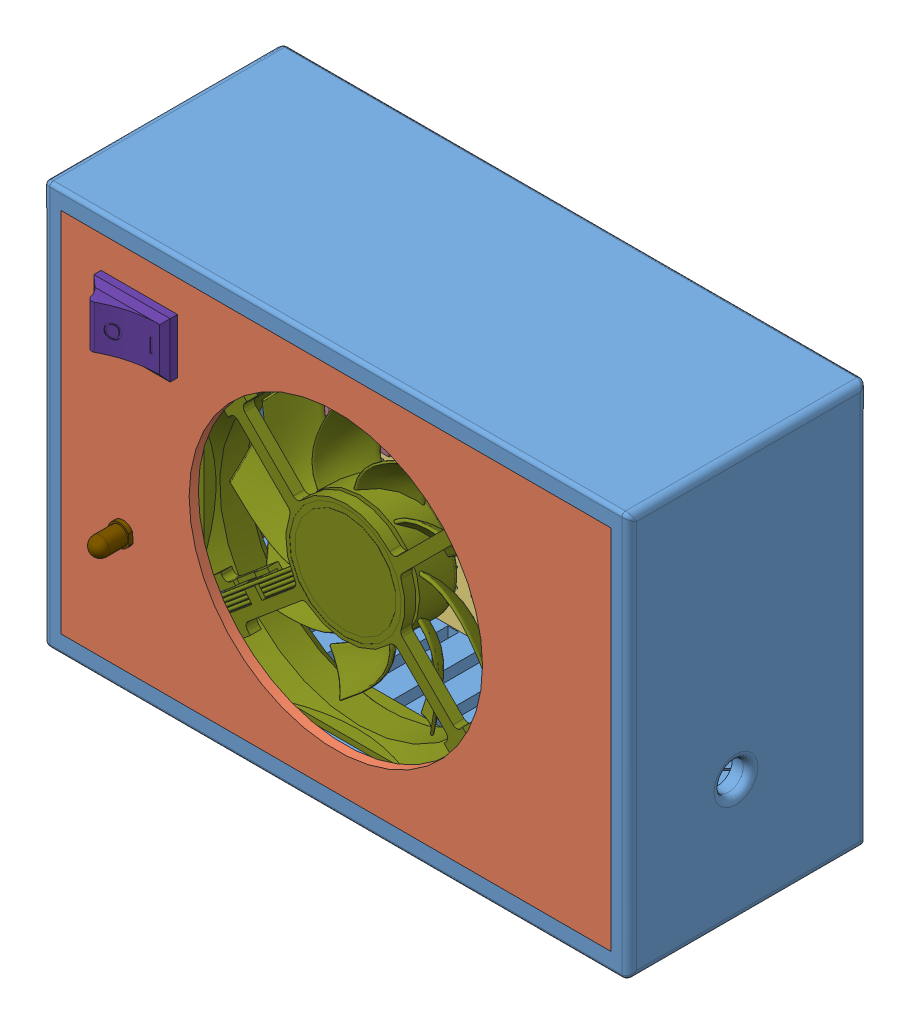
SolidWorks assembly Assem1 final, configuration Default. Lengths in mm.
Overall size (160 110 73.7).
688 component instances, 72 part files, 18 mates.
Components (placement in the parent):
- Lead acid charger_enclosure-2: Lead acid charger_enclosure [Default] at origin size (160 110 65)
- Part2-3: Part2 [Default] at (0 0 60) x (0 0 -1) z (1 0 0) size (42.25 100 150)
- PCB2.step-2: PCB2.step [Default] at (-67.4243 -42.9166 12.1575) size (119 88 45.91)
  - Board.step-1: Board.step [Default] at origin size (119 88 0.41)
    - Open CASCADE STEP translator 6.8 2.1.1.step-1: Open CASCADE STEP translator 6.8 2.1.1.step [Default] at (0 0 -0.4115) size (119 88 0.41)
  - D3.step-1: D3.step [Default] at origin size (2.72 10.58 4.72)
    - 5897140976.step-1: 5897140976.step [Default] at (24 47.5001 -2) x (0 1 0) z (0 0 1) size (2.29 2.29 1.52)
      - Cylinder.step-1: Cylinder.step [Default] at origin size (2.29 2.29 1.52)
    - 5897140736.step-1: 5897140736.step [Default] at (24 47.5001 1.36) x (0 1 0) z (0 0 1) size (0.86 0.86 0.86)
      - Sphere.step-1: Sphere.step [Default] at origin size (0.86 0.86 0.86)
    - 5897140496.step-1: 5897140496.step [Default] at (24 40.4001 1.36) x (0 0 -1) z (0 1 0) size (2.72 2.72 5.2)
      - Cylinder-0.step-1: Cylinder-0.step [Default] at origin size (2.72 2.72 5.2)
    - 5897140256.step-1: 5897140256.step [Default] at (24 45.6 1.36) x (0 0 -1) z (0 1 0) size (0.86 0.86 1.9)
      - Cylinder-1.step-1: Cylinder-1.step [Default] at origin size (0.86 0.86 1.9)
    - 5897140096.step-1: 5897140096.step [Default] at (24 40.4 1.36) x (0 0 -1) z (0 -1 0) size (0.86 0.86 1.9)
      - Cylinder-2.step-1: Cylinder-2.step [Default] at origin size (0.86 0.86 1.9)
    - 5897139936.step-1: 5897139936.step [Default] at (24 38.4999 1.36) x (0 -1 0) z (0 0 1) size (0.86 0.86 0.86)
      - Sphere-3.step-1: Sphere-3.step [Default] at origin size (0.86 0.86 0.86)
    - 5897139776.step-1: 5897139776.step [Default] at (24 38.4999 -2) x (0 -1 0) z (0 0 1) size (0.86 0.86 3.36)
      - Cylinder-4.step-1: Cylinder-4.step [Default] at origin size (0.86 0.86 3.36)
  - D1.step-1: D1.step [Default] at origin size (5.6 16.87 20.27)
    - 5790703040.step-1: 5790703040.step [Default] at (71 42 0) x (0 -1 0) z (-1 0 0) size (16.87 20.27 5.6)
  - D2.step-1: D2.step [Default] at origin size (16.87 5.6 20.27)
    - 5790703360.step-1: 5790703360.step [Default] at (79 78 0) x (-1 0 0) z (0 1 0) size (16.87 20.27 5.6)
  - U8.step-1: U8.step [Default] at origin size (7.89 10.15 6.68)
    - 5985638288.step-1: 5985638288.step [Default] at (35.891 41.689 0.51) size (6.6 10.15 4.57)
      - Extruded-5.step-1: Extruded-5.step [Default] at origin size (6.6 10.15 4.57)
    - 5985638128.step-1: 5985638128.step [Default] at (39.701 45.499 -1.6) size (0.27 0.72 1.6)
      - Extruded-2.step-1: Extruded-2.step [Default] at origin size (0.27 0.72 1.6)
    - 5985637968.step-1: 5985637968.step [Default] at (39.5135 45.499 2.66) size (0.64 1 0.27)
      - Extruded-3.step-1: Extruded-3.step [Default] at origin size (0.64 1 0.27)
    - 5985637808.step-1: 5985637808.step [Default] at (39.701 45.499 0) size (0.27 1 2.66)
      - Extruded-4.step-1: Extruded-4.step [Default] at origin size (0.27 1 2.66)
    - 5985638128.step-2: 5985638128.step [Default] at (39.701 42.959 -1.6) size (0.27 0.72 1.6)
      - Extruded-2.step-1: Extruded-2.step [Default] at origin size (0.27 0.72 1.6)
    - 5985637968.step-2: 5985637968.step [Default] at (39.5135 42.959 2.66) size (0.64 1 0.27)
      - Extruded-3.step-1: Extruded-3.step [Default] at origin size (0.64 1 0.27)
    - 5985637808.step-2: 5985637808.step [Default] at (39.701 42.959 0) size (0.27 1 2.66)
      - Extruded-4.step-1: Extruded-4.step [Default] at origin size (0.27 1 2.66)
    - 5985638128.step-3: 5985638128.step [Default] at (39.701 40.419 -1.6) size (0.27 0.72 1.6)
      - Extruded-2.step-1: Extruded-2.step [Default] at origin size (0.27 0.72 1.6)
    - 5985637968.step-3: 5985637968.step [Default] at (39.5135 40.419 2.66) size (0.64 1 0.27)
      - Extruded-3.step-1: Extruded-3.step [Default] at origin size (0.64 1 0.27)
    - 5985637808.step-3: 5985637808.step [Default] at (39.701 40.419 0) size (0.27 1 2.66)
      - Extruded-4.step-1: Extruded-4.step [Default] at origin size (0.27 1 2.66)
    - 5985638128.step-4: 5985638128.step [Default] at (39.701 37.879 -1.6) size (0.27 0.72 1.6)
      - Extruded-2.step-1: Extruded-2.step [Default] at origin size (0.27 0.72 1.6)
    - 5985637968.step-4: 5985637968.step [Default] at (39.5135 37.879 2.66) size (0.64 1 0.27)
      - Extruded-3.step-1: Extruded-3.step [Default] at origin size (0.64 1 0.27)
    - 5985637808.step-4: 5985637808.step [Default] at (39.701 37.879 0) size (0.27 1 2.66)
      - Extruded-4.step-1: Extruded-4.step [Default] at origin size (0.27 1 2.66)
    - 5985638128.step-5: 5985638128.step [Default] at (32.081 37.879 -1.6) size (0.27 0.72 1.6)
      - Extruded-2.step-1: Extruded-2.step [Default] at origin size (0.27 0.72 1.6)
    - 5985637968.step-5: 5985637968.step [Default] at (32.2685 37.879 2.66) size (0.64 1 0.27)
      - Extruded-3.step-1: Extruded-3.step [Default] at origin size (0.64 1 0.27)
    - 5985637808.step-5: 5985637808.step [Default] at (32.081 37.879 0) size (0.27 1 2.66)
      - Extruded-4.step-1: Extruded-4.step [Default] at origin size (0.27 1 2.66)
    - 5985638128.step-6: 5985638128.step [Default] at (32.081 40.419 -1.6) size (0.27 0.72 1.6)
      - Extruded-2.step-1: Extruded-2.step [Default] at origin size (0.27 0.72 1.6)
    - 5985637968.step-6: 5985637968.step [Default] at (32.2685 40.419 2.66) size (0.64 1 0.27)
      - Extruded-3.step-1: Extruded-3.step [Default] at origin size (0.64 1 0.27)
    - 5985637808.step-6: 5985637808.step [Default] at (32.081 40.419 0) size (0.27 1 2.66)
      - Extruded-4.step-1: Extruded-4.step [Default] at origin size (0.27 1 2.66)
    - 5985638128.step-7: 5985638128.step [Default] at (32.081 42.959 -1.6) size (0.27 0.72 1.6)
      - Extruded-2.step-1: Extruded-2.step [Default] at origin size (0.27 0.72 1.6)
    - 5985637968.step-7: 5985637968.step [Default] at (32.2685 42.959 2.66) size (0.64 1 0.27)
      - Extruded-3.step-1: Extruded-3.step [Default] at origin size (0.64 1 0.27)
    - 5985637808.step-7: 5985637808.step [Default] at (32.081 42.959 0) size (0.27 1 2.66)
      - Extruded-4.step-1: Extruded-4.step [Default] at origin size (0.27 1 2.66)
    - 5985638128.step-8: 5985638128.step [Default] at (32.081 45.499 -1.6) size (0.27 0.72 1.6)
      - Extruded-2.step-1: Extruded-2.step [Default] at origin size (0.27 0.72 1.6)
    - 5985637968.step-8: 5985637968.step [Default] at (32.2685 45.499 2.66) size (0.64 1 0.27)
      - Extruded-3.step-1: Extruded-3.step [Default] at origin size (0.64 1 0.27)
    - 5985637808.step-8: 5985637808.step [Default] at (32.081 45.499 0) size (0.27 1 2.66)
      - Extruded-4.step-1: Extruded-4.step [Default] at origin size (0.27 1 2.66)
  - U9.step-1: U9.step [Default] at origin size (7.89 19.7 6.68)
    - 5985054240.step-1: 5985054240.step [Default] at (35.764 14.13 0.51) size (6.6 19.7 4.57)
      - Extruded-1.step-1: Extruded-1.step [Default] at origin size (6.6 19.7 4.57)
    - 5985638128.step-1: 5985638128.step [Default] at (39.574 23.02 -1.6) size (0.27 0.72 1.6)
      - Extruded-2.step-1: Extruded-2.step [Default] at origin size (0.27 0.72 1.6)
    - 5985637968.step-1: 5985637968.step [Default] at (39.3865 23.02 2.66) size (0.64 1 0.27)
      - Extruded-3.step-1: Extruded-3.step [Default] at origin size (0.64 1 0.27)
    - 5985637808.step-1: 5985637808.step [Default] at (39.574 23.02 0) size (0.27 1 2.66)
      - Extruded-4.step-1: Extruded-4.step [Default] at origin size (0.27 1 2.66)
    - 5985638128.step-2: 5985638128.step [Default] at (39.574 20.48 -1.6) size (0.27 0.72 1.6)
      - Extruded-2.step-1: Extruded-2.step [Default] at origin size (0.27 0.72 1.6)
    - 5985637968.step-2: 5985637968.step [Default] at (39.3865 20.48 2.66) size (0.64 1 0.27)
      - Extruded-3.step-1: Extruded-3.step [Default] at origin size (0.64 1 0.27)
    - 5985637808.step-2: 5985637808.step [Default] at (39.574 20.48 0) size (0.27 1 2.66)
      - Extruded-4.step-1: Extruded-4.step [Default] at origin size (0.27 1 2.66)
    - 5985638128.step-3: 5985638128.step [Default] at (39.574 17.94 -1.6) size (0.27 0.72 1.6)
      - Extruded-2.step-1: Extruded-2.step [Default] at origin size (0.27 0.72 1.6)
    - 5985637968.step-3: 5985637968.step [Default] at (39.3865 17.94 2.66) size (0.64 1 0.27)
      - Extruded-3.step-1: Extruded-3.step [Default] at origin size (0.64 1 0.27)
    - 5985637808.step-3: 5985637808.step [Default] at (39.574 17.94 0) size (0.27 1 2.66)
      - Extruded-4.step-1: Extruded-4.step [Default] at origin size (0.27 1 2.66)
    - 5985638128.step-4: 5985638128.step [Default] at (39.574 15.4 -1.6) size (0.27 0.72 1.6)
      - Extruded-2.step-1: Extruded-2.step [Default] at origin size (0.27 0.72 1.6)
    - 5985637968.step-4: 5985637968.step [Default] at (39.3865 15.4 2.66) size (0.64 1 0.27)
      - Extruded-3.step-1: Extruded-3.step [Default] at origin size (0.64 1 0.27)
    - 5985637808.step-4: 5985637808.step [Default] at (39.574 15.4 0) size (0.27 1 2.66)
      - Extruded-4.step-1: Extruded-4.step [Default] at origin size (0.27 1 2.66)
    - 5985638128.step-5: 5985638128.step [Default] at (39.574 12.86 -1.6) size (0.27 0.72 1.6)
      - Extruded-2.step-1: Extruded-2.step [Default] at origin size (0.27 0.72 1.6)
    - 5985637968.step-5: 5985637968.step [Default] at (39.3865 12.86 2.66) size (0.64 1 0.27)
      - Extruded-3.step-1: Extruded-3.step [Default] at origin size (0.64 1 0.27)
    - 5985637808.step-5: 5985637808.step [Default] at (39.574 12.86 0) size (0.27 1 2.66)
      - Extruded-4.step-1: Extruded-4.step [Default] at origin size (0.27 1 2.66)
    - 5985638128.step-6: 5985638128.step [Default] at (39.574 10.32 -1.6) size (0.27 0.72 1.6)
      - Extruded-2.step-1: Extruded-2.step [Default] at origin size (0.27 0.72 1.6)
    - 5985637968.step-6: 5985637968.step [Default] at (39.3865 10.32 2.66) size (0.64 1 0.27)
      - Extruded-3.step-1: Extruded-3.step [Default] at origin size (0.64 1 0.27)
    - 5985637808.step-6: 5985637808.step [Default] at (39.574 10.32 0) size (0.27 1 2.66)
      - Extruded-4.step-1: Extruded-4.step [Default] at origin size (0.27 1 2.66)
    - 5985638128.step-7: 5985638128.step [Default] at (39.574 7.78 -1.6) size (0.27 0.72 1.6)
      - Extruded-2.step-1: Extruded-2.step [Default] at origin size (0.27 0.72 1.6)
    - 5985637968.step-7: 5985637968.step [Default] at (39.3865 7.78 2.66) size (0.64 1 0.27)
      - Extruded-3.step-1: Extruded-3.step [Default] at origin size (0.64 1 0.27)
    - 5985637808.step-7: 5985637808.step [Default] at (39.574 7.78 0) size (0.27 1 2.66)
      - Extruded-4.step-1: Extruded-4.step [Default] at origin size (0.27 1 2.66)
    - 5985638128.step-8: 5985638128.step [Default] at (39.574 5.24 -1.6) size (0.27 0.72 1.6)
      - Extruded-2.step-1: Extruded-2.step [Default] at origin size (0.27 0.72 1.6)
    - 5985637968.step-8: 5985637968.step [Default] at (39.3865 5.24 2.66) size (0.64 1 0.27)
      - Extruded-3.step-1: Extruded-3.step [Default] at origin size (0.64 1 0.27)
    - 5985637808.step-8: 5985637808.step [Default] at (39.574 5.24 0) size (0.27 1 2.66)
      - Extruded-4.step-1: Extruded-4.step [Default] at origin size (0.27 1 2.66)
    - 5985638128.step-9: 5985638128.step [Default] at (31.954 5.24 -1.6) size (0.27 0.72 1.6)
      - Extruded-2.step-1: Extruded-2.step [Default] at origin size (0.27 0.72 1.6)
    - 5985637968.step-9: 5985637968.step [Default] at (32.1415 5.24 2.66) size (0.64 1 0.27)
      - Extruded-3.step-1: Extruded-3.step [Default] at origin size (0.64 1 0.27)
    - 5985637808.step-9: 5985637808.step [Default] at (31.954 5.24 0) size (0.27 1 2.66)
      - Extruded-4.step-1: Extruded-4.step [Default] at origin size (0.27 1 2.66)
    - 5985638128.step-10: 5985638128.step [Default] at (31.954 7.78 -1.6) size (0.27 0.72 1.6)
      - Extruded-2.step-1: Extruded-2.step [Default] at origin size (0.27 0.72 1.6)
    - 5985637968.step-10: 5985637968.step [Default] at (32.1415 7.78 2.66) size (0.64 1 0.27)
      - Extruded-3.step-1: Extruded-3.step [Default] at origin size (0.64 1 0.27)
    - 5985637808.step-10: 5985637808.step [Default] at (31.954 7.78 0) size (0.27 1 2.66)
      - Extruded-4.step-1: Extruded-4.step [Default] at origin size (0.27 1 2.66)
    - 5985638128.step-11: 5985638128.step [Default] at (31.954 10.32 -1.6) size (0.27 0.72 1.6)
      - Extruded-2.step-1: Extruded-2.step [Default] at origin size (0.27 0.72 1.6)
    - 5985637968.step-11: 5985637968.step [Default] at (32.1415 10.32 2.66) size (0.64 1 0.27)
      - Extruded-3.step-1: Extruded-3.step [Default] at origin size (0.64 1 0.27)
    - 5985637808.step-11: 5985637808.step [Default] at (31.954 10.32 0) size (0.27 1 2.66)
      - Extruded-4.step-1: Extruded-4.step [Default] at origin size (0.27 1 2.66)
    - 5985638128.step-12: 5985638128.step [Default] at (31.954 12.86 -1.6) size (0.27 0.72 1.6)
      - Extruded-2.step-1: Extruded-2.step [Default] at origin size (0.27 0.72 1.6)
    - 5985637968.step-12: 5985637968.step [Default] at (32.1415 12.86 2.66) size (0.64 1 0.27)
      - Extruded-3.step-1: Extruded-3.step [Default] at origin size (0.64 1 0.27)
    - 5985637808.step-12: 5985637808.step [Default] at (31.954 12.86 0) size (0.27 1 2.66)
      - Extruded-4.step-1: Extruded-4.step [Default] at origin size (0.27 1 2.66)
    - 5985638128.step-13: 5985638128.step [Default] at (31.954 15.4 -1.6) size (0.27 0.72 1.6)
      - Extruded-2.step-1: Extruded-2.step [Default] at origin size (0.27 0.72 1.6)
    - 5985637968.step-13: 5985637968.step [Default] at (32.1415 15.4 2.66) size (0.64 1 0.27)
      - Extruded-3.step-1: Extruded-3.step [Default] at origin size (0.64 1 0.27)
    - 5985637808.step-13: 5985637808.step [Default] at (31.954 15.4 0) size (0.27 1 2.66)
      - Extruded-4.step-1: Extruded-4.step [Default] at origin size (0.27 1 2.66)
    - 5985638128.step-14: 5985638128.step [Default] at (31.954 17.94 -1.6) size (0.27 0.72 1.6)
      - Extruded-2.step-1: Extruded-2.step [Default] at origin size (0.27 0.72 1.6)
    - 5985637968.step-14: 5985637968.step [Default] at (32.1415 17.94 2.66) size (0.64 1 0.27)
      - Extruded-3.step-1: Extruded-3.step [Default] at origin size (0.64 1 0.27)
    - 5985637808.step-14: 5985637808.step [Default] at (31.954 17.94 0) size (0.27 1 2.66)
      - Extruded-4.step-1: Extruded-4.step [Default] at origin size (0.27 1 2.66)
    - 5985638128.step-15: 5985638128.step [Default] at (31.954 20.48 -1.6) size (0.27 0.72 1.6)
      - Extruded-2.step-1: Extruded-2.step [Default] at origin size (0.27 0.72 1.6)
    - 5985637968.step-15: 5985637968.step [Default] at (32.1415 20.48 2.66) size (0.64 1 0.27)
      - Extruded-3.step-1: Extruded-3.step [Default] at origin size (0.64 1 0.27)
    - 5985637808.step-15: 5985637808.step [Default] at (31.954 20.48 0) size (0.27 1 2.66)
      - Extruded-4.step-1: Extruded-4.step [Default] at origin size (0.27 1 2.66)
    - 5985638128.step-16: 5985638128.step [Default] at (31.954 23.02 -1.6) size (0.27 0.72 1.6)
      - Extruded-2.step-1: Extruded-2.step [Default] at origin size (0.27 0.72 1.6)
    - 5985637968.step-16: 5985637968.step [Default] at (32.1415 23.02 2.66) size (0.64 1 0.27)
      - Extruded-3.step-1: Extruded-3.step [Default] at origin size (0.64 1 0.27)
    - 5985637808.step-16: 5985637808.step [Default] at (31.954 23.02 0) size (0.27 1 2.66)
      - Extruded-4.step-1: Extruded-4.step [Default] at origin size (0.27 1 2.66)
  - U3.step-1: U3.step [Default] at origin size (7.89 10.15 6.68)
    - 5985637808.step-1: 5985637808.step [Default] at (38.8016 79.789 0) size (0.27 1 2.66)
      - Extruded-4.step-1: Extruded-4.step [Default] at origin size (0.27 1 2.66)
    - 5985637968.step-1: 5985637968.step [Default] at (38.9891 79.789 2.66) size (0.64 1 0.27)
      - Extruded-3.step-1: Extruded-3.step [Default] at origin size (0.64 1 0.27)
    - 5985638128.step-1: 5985638128.step [Default] at (38.8016 79.789 -1.6) size (0.27 0.72 1.6)
      - Extruded-2.step-1: Extruded-2.step [Default] at origin size (0.27 0.72 1.6)
    - 5985637808.step-2: 5985637808.step [Default] at (38.8016 77.249 0) size (0.27 1 2.66)
      - Extruded-4.step-1: Extruded-4.step [Default] at origin size (0.27 1 2.66)
    - 5985637968.step-2: 5985637968.step [Default] at (38.9891 77.249 2.66) size (0.64 1 0.27)
      - Extruded-3.step-1: Extruded-3.step [Default] at origin size (0.64 1 0.27)
    - 5985638128.step-2: 5985638128.step [Default] at (38.8016 77.249 -1.6) size (0.27 0.72 1.6)
      - Extruded-2.step-1: Extruded-2.step [Default] at origin size (0.27 0.72 1.6)
    - 5985637808.step-3: 5985637808.step [Default] at (38.8016 74.709 0) size (0.27 1 2.66)
      - Extruded-4.step-1: Extruded-4.step [Default] at origin size (0.27 1 2.66)
    - 5985637968.step-3: 5985637968.step [Default] at (38.9891 74.709 2.66) size (0.64 1 0.27)
      - Extruded-3.step-1: Extruded-3.step [Default] at origin size (0.64 1 0.27)
    - 5985638128.step-3: 5985638128.step [Default] at (38.8016 74.709 -1.6) size (0.27 0.72 1.6)
      - Extruded-2.step-1: Extruded-2.step [Default] at origin size (0.27 0.72 1.6)
    - 5985637808.step-4: 5985637808.step [Default] at (38.8016 72.169 0) size (0.27 1 2.66)
      - Extruded-4.step-1: Extruded-4.step [Default] at origin size (0.27 1 2.66)
    - 5985637968.step-4: 5985637968.step [Default] at (38.9891 72.169 2.66) size (0.64 1 0.27)
      - Extruded-3.step-1: Extruded-3.step [Default] at origin size (0.64 1 0.27)
    - 5985638128.step-4: 5985638128.step [Default] at (38.8016 72.169 -1.6) size (0.27 0.72 1.6)
      - Extruded-2.step-1: Extruded-2.step [Default] at origin size (0.27 0.72 1.6)
    - 5985637808.step-5: 5985637808.step [Default] at (46.4216 72.169 0) size (0.27 1 2.66)
      - Extruded-4.step-1: Extruded-4.step [Default] at origin size (0.27 1 2.66)
    - 5985637968.step-5: 5985637968.step [Default] at (46.2341 72.169 2.66) size (0.64 1 0.27)
      - Extruded-3.step-1: Extruded-3.step [Default] at origin size (0.64 1 0.27)
    - 5985638128.step-5: 5985638128.step [Default] at (46.4216 72.169 -1.6) size (0.27 0.72 1.6)
      - Extruded-2.step-1: Extruded-2.step [Default] at origin size (0.27 0.72 1.6)
    - 5985637808.step-6: 5985637808.step [Default] at (46.4216 74.709 0) size (0.27 1 2.66)
      - Extruded-4.step-1: Extruded-4.step [Default] at origin size (0.27 1 2.66)
    - 5985637968.step-6: 5985637968.step [Default] at (46.2341 74.709 2.66) size (0.64 1 0.27)
      - Extruded-3.step-1: Extruded-3.step [Default] at origin size (0.64 1 0.27)
    - 5985638128.step-6: 5985638128.step [Default] at (46.4216 74.709 -1.6) size (0.27 0.72 1.6)
      - Extruded-2.step-1: Extruded-2.step [Default] at origin size (0.27 0.72 1.6)
    - 5985637808.step-7: 5985637808.step [Default] at (46.4216 77.249 0) size (0.27 1 2.66)
      - Extruded-4.step-1: Extruded-4.step [Default] at origin size (0.27 1 2.66)
    - 5985637968.step-7: 5985637968.step [Default] at (46.2341 77.249 2.66) size (0.64 1 0.27)
      - Extruded-3.step-1: Extruded-3.step [Default] at origin size (0.64 1 0.27)
    - 5985638128.step-7: 5985638128.step [Default] at (46.4216 77.249 -1.6) size (0.27 0.72 1.6)
      - Extruded-2.step-1: Extruded-2.step [Default] at origin size (0.27 0.72 1.6)
    - 5985637808.step-8: 5985637808.step [Default] at (46.4216 79.789 0) size (0.27 1 2.66)
      - Extruded-4.step-1: Extruded-4.step [Default] at origin size (0.27 1 2.66)
    - 5985637968.step-8: 5985637968.step [Default] at (46.2341 79.789 2.66) size (0.64 1 0.27)
      - Extruded-3.step-1: Extruded-3.step [Default] at origin size (0.64 1 0.27)
    - 5985638128.step-8: 5985638128.step [Default] at (46.4216 79.789 -1.6) size (0.27 0.72 1.6)
      - Extruded-2.step-1: Extruded-2.step [Default] at origin size (0.27 0.72 1.6)
    - 5985638288.step-1: 5985638288.step [Default] at (42.6116 75.979 0.51) size (6.6 10.15 4.57)
      - Extruded-5.step-1: Extruded-5.step [Default] at origin size (6.6 10.15 4.57)
  - R5.step-1: R5.step [Default] at origin size (29.91 9.5 14)
    - Res_Yageo_SQP500JB-1R2_eec.step-1: Res_Yageo_SQP500JB-1R2_eec.step [Default] at (102 46 0) x (-1 0 0) z (0 0 1) size (29.91 9.5 14)
      - 1.step-1: 1.step [Default] at origin size (29.91 0.8 9.4)
      - 2.step-1: 2.step [Default] at origin size (22 9.5 10)
      - Yageo_Logo.step-1: Yageo_Logo.step [Default] at (-8.1443 3.6121 9.991) size (4.52 1.05 0.01)
  - R6_B.step-1: R6_B.step [Default] at origin size (9.5 29.91 14)
    - Res_Yageo_SQP500JB-1R2_eec.step-1: Res_Yageo_SQP500JB-1R2_eec.step [Default] at (112 21 0) x (0 1 0) z (0 0 1) size (29.91 9.5 14)
      - 1.step-1: 1.step [Default] at origin size (29.91 0.8 9.4)
      - 2.step-1: 2.step [Default] at origin size (22 9.5 10)
      - Yageo_Logo.step-1: Yageo_Logo.step [Default] at (-8.1443 3.6121 9.991) size (4.52 1.05 0.01)
  - J3.step-1: J3.step [Default] at origin size (10.16 4.2 31.24)
    - 5878482320.step-1: 5878482320.step [Default] at (85 57 0) x (1 0 0) z (0 -1 0) size (10.16 31.24 4.2)
  - VRV.step-1: VRV.step [Default] at origin size (6.6 6.99 4.95)
    - 5985046800.step-1: 5985046800.step [Default] at (48.0794 28.192 0) size (6.6 6.99 4.95)
      - Extruded-0.step-1: Extruded-0.step [Default] at origin size (6.6 6.99 4.95)
  - VR.step-1: VR.step [Default] at origin size (6.6 6.99 4.95)
    - 5985046800.step-1: 5985046800.step [Default] at (14.428 36.99 0) size (6.6 6.99 4.95)
      - Extruded-0.step-1: Extruded-0.step [Default] at origin size (6.6 6.99 4.95)
  - VRC.step-1: VRC.step [Default] at origin size (6.6 6.99 4.95)
    - 5985046800.step-1: 5985046800.step [Default] at (61.031 28.192 0) size (6.6 6.99 4.95)
      - Extruded-0.step-1: Extruded-0.step [Default] at origin size (6.6 6.99 4.95)
  - U7.step-1: U7.step [Default] at origin size (7.89 19.7 6.68)
    - 5985054240.step-1: 5985054240.step [Default] at (22.81 14.62 0.51) size (6.6 19.7 4.57)
      - Extruded-1.step-1: Extruded-1.step [Default] at origin size (6.6 19.7 4.57)
    - 5985638128.step-1: 5985638128.step [Default] at (26.62 22.24 -1.6) size (0.27 0.72 1.6)
      - Extruded-2.step-1: Extruded-2.step [Default] at origin size (0.27 0.72 1.6)
    - 5985637968.step-1: 5985637968.step [Default] at (26.4325 22.24 2.66) size (0.64 1 0.27)
      - Extruded-3.step-1: Extruded-3.step [Default] at origin size (0.64 1 0.27)
    - 5985637808.step-1: 5985637808.step [Default] at (26.62 22.24 0) size (0.27 1 2.66)
      - Extruded-4.step-1: Extruded-4.step [Default] at origin size (0.27 1 2.66)
    - 5985638128.step-2: 5985638128.step [Default] at (26.62 19.7 -1.6) size (0.27 0.72 1.6)
      - Extruded-2.step-1: Extruded-2.step [Default] at origin size (0.27 0.72 1.6)
    - 5985637968.step-2: 5985637968.step [Default] at (26.4325 19.7 2.66) size (0.64 1 0.27)
      - Extruded-3.step-1: Extruded-3.step [Default] at origin size (0.64 1 0.27)
    - 5985637808.step-2: 5985637808.step [Default] at (26.62 19.7 0) size (0.27 1 2.66)
      - Extruded-4.step-1: Extruded-4.step [Default] at origin size (0.27 1 2.66)
    - 5985638128.step-3: 5985638128.step [Default] at (26.62 17.16 -1.6) size (0.27 0.72 1.6)
      - Extruded-2.step-1: Extruded-2.step [Default] at origin size (0.27 0.72 1.6)
    - 5985637968.step-3: 5985637968.step [Default] at (26.4325 17.16 2.66) size (0.64 1 0.27)
      - Extruded-3.step-1: Extruded-3.step [Default] at origin size (0.64 1 0.27)
    - 5985637808.step-3: 5985637808.step [Default] at (26.62 17.16 0) size (0.27 1 2.66)
      - Extruded-4.step-1: Extruded-4.step [Default] at origin size (0.27 1 2.66)
    - 5985638128.step-4: 5985638128.step [Default] at (26.62 14.62 -1.6) size (0.27 0.72 1.6)
      - Extruded-2.step-1: Extruded-2.step [Default] at origin size (0.27 0.72 1.6)
    - 5985637968.step-4: 5985637968.step [Default] at (26.4325 14.62 2.66) size (0.64 1 0.27)
      - Extruded-3.step-1: Extruded-3.step [Default] at origin size (0.64 1 0.27)
    - 5985637808.step-4: 5985637808.step [Default] at (26.62 14.62 0) size (0.27 1 2.66)
      - Extruded-4.step-1: Extruded-4.step [Default] at origin size (0.27 1 2.66)
    - 5985638128.step-5: 5985638128.step [Default] at (26.62 12.08 -1.6) size (0.27 0.72 1.6)
      - Extruded-2.step-1: Extruded-2.step [Default] at origin size (0.27 0.72 1.6)
    - 5985637968.step-5: 5985637968.step [Default] at (26.4325 12.08 2.66) size (0.64 1 0.27)
      - Extruded-3.step-1: Extruded-3.step [Default] at origin size (0.64 1 0.27)
    - 5985637808.step-5: 5985637808.step [Default] at (26.62 12.08 0) size (0.27 1 2.66)
      - Extruded-4.step-1: Extruded-4.step [Default] at origin size (0.27 1 2.66)
    - 5985638128.step-6: 5985638128.step [Default] at (26.62 9.54 -1.6) size (0.27 0.72 1.6)
      - Extruded-2.step-1: Extruded-2.step [Default] at origin size (0.27 0.72 1.6)
    - 5985637968.step-6: 5985637968.step [Default] at (26.4325 9.54 2.66) size (0.64 1 0.27)
      - Extruded-3.step-1: Extruded-3.step [Default] at origin size (0.64 1 0.27)
    - 5985637808.step-6: 5985637808.step [Default] at (26.62 9.54 0) size (0.27 1 2.66)
      - Extruded-4.step-1: Extruded-4.step [Default] at origin size (0.27 1 2.66)
    - 5985638128.step-7: 5985638128.step [Default] at (26.62 7 -1.6) size (0.27 0.72 1.6)
      - Extruded-2.step-1: Extruded-2.step [Default] at origin size (0.27 0.72 1.6)
    - 5985637968.step-7: 5985637968.step [Default] at (26.4325 7 2.66) size (0.64 1 0.27)
      - Extruded-3.step-1: Extruded-3.step [Default] at origin size (0.64 1 0.27)
    - 5985637808.step-7: 5985637808.step [Default] at (26.62 7 0) size (0.27 1 2.66)
      - Extruded-4.step-1: Extruded-4.step [Default] at origin size (0.27 1 2.66)
    - 5985638128.step-8: 5985638128.step [Default] at (19 7 -1.6) size (0.27 0.72 1.6)
      - Extruded-2.step-1: Extruded-2.step [Default] at origin size (0.27 0.72 1.6)
    - 5985637968.step-8: 5985637968.step [Default] at (19.1875 7 2.66) size (0.64 1 0.27)
      - Extruded-3.step-1: Extruded-3.step [Default] at origin size (0.64 1 0.27)
    - 5985637808.step-8: 5985637808.step [Default] at (19 7 0) size (0.27 1 2.66)
      - Extruded-4.step-1: Extruded-4.step [Default] at origin size (0.27 1 2.66)
    - 5985638128.step-9: 5985638128.step [Default] at (19 9.54 -1.6) size (0.27 0.72 1.6)
      - Extruded-2.step-1: Extruded-2.step [Default] at origin size (0.27 0.72 1.6)
    - 5985637968.step-9: 5985637968.step [Default] at (19.1875 9.54 2.66) size (0.64 1 0.27)
      - Extruded-3.step-1: Extruded-3.step [Default] at origin size (0.64 1 0.27)
    - 5985637808.step-9: 5985637808.step [Default] at (19 9.54 0) size (0.27 1 2.66)
      - Extruded-4.step-1: Extruded-4.step [Default] at origin size (0.27 1 2.66)
    - 5985638128.step-10: 5985638128.step [Default] at (19 12.08 -1.6) size (0.27 0.72 1.6)
      - Extruded-2.step-1: Extruded-2.step [Default] at origin size (0.27 0.72 1.6)
    - 5985637968.step-10: 5985637968.step [Default] at (19.1875 12.08 2.66) size (0.64 1 0.27)
      - Extruded-3.step-1: Extruded-3.step [Default] at origin size (0.64 1 0.27)
    - 5985637808.step-10: 5985637808.step [Default] at (19 12.08 0) size (0.27 1 2.66)
      - Extruded-4.step-1: Extruded-4.step [Default] at origin size (0.27 1 2.66)
    - 5985638128.step-11: 5985638128.step [Default] at (19 14.62 -1.6) size (0.27 0.72 1.6)
      - Extruded-2.step-1: Extruded-2.step [Default] at origin size (0.27 0.72 1.6)
    - 5985637968.step-11: 5985637968.step [Default] at (19.1875 14.62 2.66) size (0.64 1 0.27)
      - Extruded-3.step-1: Extruded-3.step [Default] at origin size (0.64 1 0.27)
    - 5985637808.step-11: 5985637808.step [Default] at (19 14.62 0) size (0.27 1 2.66)
      - Extruded-4.step-1: Extruded-4.step [Default] at origin size (0.27 1 2.66)
    - 5985638128.step-12: 5985638128.step [Default] at (19 17.16 -1.6) size (0.27 0.72 1.6)
      - Extruded-2.step-1: Extruded-2.step [Default] at origin size (0.27 0.72 1.6)
    - 5985637968.step-12: 5985637968.step [Default] at (19.1875 17.16 2.66) size (0.64 1 0.27)
      - Extruded-3.step-1: Extruded-3.step [Default] at origin size (0.64 1 0.27)
    - 5985637808.step-12: 5985637808.step [Default] at (19 17.16 0) size (0.27 1 2.66)
      - Extruded-4.step-1: Extruded-4.step [Default] at origin size (0.27 1 2.66)
    - 5985638128.step-13: 5985638128.step [Default] at (19 19.7 -1.6) size (0.27 0.72 1.6)
      - Extruded-2.step-1: Extruded-2.step [Default] at origin size (0.27 0.72 1.6)
    - 5985637968.step-13: 5985637968.step [Default] at (19.1875 19.7 2.66) size (0.64 1 0.27)
      - Extruded-3.step-1: Extruded-3.step [Default] at origin size (0.64 1 0.27)
    - 5985637808.step-13: 5985637808.step [Default] at (19 19.7 0) size (0.27 1 2.66)
      - Extruded-4.step-1: Extruded-4.step [Default] at origin size (0.27 1 2.66)
    - 5985638128.step-14: 5985638128.step [Default] at (19 22.24 -1.6) size (0.27 0.72 1.6)
      - Extruded-2.step-1: Extruded-2.step [Default] at origin size (0.27 0.72 1.6)
    - 5985637968.step-14: 5985637968.step [Default] at (19.1875 22.24 2.66) size (0.64 1 0.27)
      - Extruded-3.step-1: Extruded-3.step [Default] at origin size (0.64 1 0.27)
    - 5985637808.step-14: 5985637808.step [Default] at (19 22.24 0) size (0.27 1 2.66)
      - Extruded-4.step-1: Extruded-4.step [Default] at origin size (0.27 1 2.66)
  - U6.step-1: U6.step [Default] at origin size (7.89 10.15 6.68)
    - 5985638288.step-1: 5985638288.step [Default] at (48.591 41.689 0.51) size (6.6 10.15 4.57)
      - Extruded-5.step-1: Extruded-5.step [Default] at origin size (6.6 10.15 4.57)
    - 5985638128.step-1: 5985638128.step [Default] at (52.401 45.499 -1.6) size (0.27 0.72 1.6)
      - Extruded-2.step-1: Extruded-2.step [Default] at origin size (0.27 0.72 1.6)
    - 5985637968.step-1: 5985637968.step [Default] at (52.2135 45.499 2.66) size (0.64 1 0.27)
      - Extruded-3.step-1: Extruded-3.step [Default] at origin size (0.64 1 0.27)
    - 5985637808.step-1: 5985637808.step [Default] at (52.401 45.499 0) size (0.27 1 2.66)
      - Extruded-4.step-1: Extruded-4.step [Default] at origin size (0.27 1 2.66)
    - 5985638128.step-2: 5985638128.step [Default] at (52.401 42.959 -1.6) size (0.27 0.72 1.6)
      - Extruded-2.step-1: Extruded-2.step [Default] at origin size (0.27 0.72 1.6)
    - 5985637968.step-2: 5985637968.step [Default] at (52.2135 42.959 2.66) size (0.64 1 0.27)
      - Extruded-3.step-1: Extruded-3.step [Default] at origin size (0.64 1 0.27)
    - 5985637808.step-2: 5985637808.step [Default] at (52.401 42.959 0) size (0.27 1 2.66)
      - Extruded-4.step-1: Extruded-4.step [Default] at origin size (0.27 1 2.66)
    - 5985638128.step-3: 5985638128.step [Default] at (52.401 40.419 -1.6) size (0.27 0.72 1.6)
      - Extruded-2.step-1: Extruded-2.step [Default] at origin size (0.27 0.72 1.6)
    - 5985637968.step-3: 5985637968.step [Default] at (52.2135 40.419 2.66) size (0.64 1 0.27)
      - Extruded-3.step-1: Extruded-3.step [Default] at origin size (0.64 1 0.27)
    - 5985637808.step-3: 5985637808.step [Default] at (52.401 40.419 0) size (0.27 1 2.66)
      - Extruded-4.step-1: Extruded-4.step [Default] at origin size (0.27 1 2.66)
    - 5985638128.step-4: 5985638128.step [Default] at (52.401 37.879 -1.6) size (0.27 0.72 1.6)
      - Extruded-2.step-1: Extruded-2.step [Default] at origin size (0.27 0.72 1.6)
    - 5985637968.step-4: 5985637968.step [Default] at (52.2135 37.879 2.66) size (0.64 1 0.27)
      - Extruded-3.step-1: Extruded-3.step [Default] at origin size (0.64 1 0.27)
    - 5985637808.step-4: 5985637808.step [Default] at (52.401 37.879 0) size (0.27 1 2.66)
      - Extruded-4.step-1: Extruded-4.step [Default] at origin size (0.27 1 2.66)
    - 5985638128.step-5: 5985638128.step [Default] at (44.781 37.879 -1.6) size (0.27 0.72 1.6)
      - Extruded-2.step-1: Extruded-2.step [Default] at origin size (0.27 0.72 1.6)
    - 5985637968.step-5: 5985637968.step [Default] at (44.9685 37.879 2.66) size (0.64 1 0.27)
      - Extruded-3.step-1: Extruded-3.step [Default] at origin size (0.64 1 0.27)
    - 5985637808.step-5: 5985637808.step [Default] at (44.781 37.879 0) size (0.27 1 2.66)
      - Extruded-4.step-1: Extruded-4.step [Default] at origin size (0.27 1 2.66)
    - 5985638128.step-6: 5985638128.step [Default] at (44.781 40.419 -1.6) size (0.27 0.72 1.6)
      - Extruded-2.step-1: Extruded-2.step [Default] at origin size (0.27 0.72 1.6)
    - 5985637968.step-6: 5985637968.step [Default] at (44.9685 40.419 2.66) size (0.64 1 0.27)
      - Extruded-3.step-1: Extruded-3.step [Default] at origin size (0.64 1 0.27)
    - 5985637808.step-6: 5985637808.step [Default] at (44.781 40.419 0) size (0.27 1 2.66)
      - Extruded-4.step-1: Extruded-4.step [Default] at origin size (0.27 1 2.66)
    - 5985638128.step-7: 5985638128.step [Default] at (44.781 42.959 -1.6) size (0.27 0.72 1.6)
      - Extruded-2.step-1: Extruded-2.step [Default] at origin size (0.27 0.72 1.6)
    - 5985637968.step-7: 5985637968.step [Default] at (44.9685 42.959 2.66) size (0.64 1 0.27)
      - Extruded-3.step-1: Extruded-3.step [Default] at origin size (0.64 1 0.27)
    - 5985637808.step-7: 5985637808.step [Default] at (44.781 42.959 0) size (0.27 1 2.66)
      - Extruded-4.step-1: Extruded-4.step [Default] at origin size (0.27 1 2.66)
    - 5985638128.step-8: 5985638128.step [Default] at (44.781 45.499 -1.6) size (0.27 0.72 1.6)
      - Extruded-2.step-1: Extruded-2.step [Default] at origin size (0.27 0.72 1.6)
    - 5985637968.step-8: 5985637968.step [Default] at (44.9685 45.499 2.66) size (0.64 1 0.27)
      - Extruded-3.step-1: Extruded-3.step [Default] at origin size (0.64 1 0.27)
    - 5985637808.step-8: 5985637808.step [Default] at (44.781 45.499 0) size (0.27 1 2.66)
      - Extruded-4.step-1: Extruded-4.step [Default] at origin size (0.27 1 2.66)
  - U5.step-1: U5.step [Default] at origin size (7.89 10.15 6.68)
    - 5985637808.step-1: 5985637808.step [Default] at (56.846 45.499 0) size (0.27 1 2.66)
      - Extruded-4.step-1: Extruded-4.step [Default] at origin size (0.27 1 2.66)
    - 5985637968.step-1: 5985637968.step [Default] at (57.0335 45.499 2.66) size (0.64 1 0.27)
      - Extruded-3.step-1: Extruded-3.step [Default] at origin size (0.64 1 0.27)
    - 5985638128.step-1: 5985638128.step [Default] at (56.846 45.499 -1.6) size (0.27 0.72 1.6)
      - Extruded-2.step-1: Extruded-2.step [Default] at origin size (0.27 0.72 1.6)
    - 5985637808.step-2: 5985637808.step [Default] at (56.846 42.959 0) size (0.27 1 2.66)
      - Extruded-4.step-1: Extruded-4.step [Default] at origin size (0.27 1 2.66)
    - 5985637968.step-2: 5985637968.step [Default] at (57.0335 42.959 2.66) size (0.64 1 0.27)
      - Extruded-3.step-1: Extruded-3.step [Default] at origin size (0.64 1 0.27)
    - 5985638128.step-2: 5985638128.step [Default] at (56.846 42.959 -1.6) size (0.27 0.72 1.6)
      - Extruded-2.step-1: Extruded-2.step [Default] at origin size (0.27 0.72 1.6)
    - 5985637808.step-3: 5985637808.step [Default] at (56.846 40.419 0) size (0.27 1 2.66)
      - Extruded-4.step-1: Extruded-4.step [Default] at origin size (0.27 1 2.66)
    - 5985637968.step-3: 5985637968.step [Default] at (57.0335 40.419 2.66) size (0.64 1 0.27)
      - Extruded-3.step-1: Extruded-3.step [Default] at origin size (0.64 1 0.27)
    - 5985638128.step-3: 5985638128.step [Default] at (56.846 40.419 -1.6) size (0.27 0.72 1.6)
      - Extruded-2.step-1: Extruded-2.step [Default] at origin size (0.27 0.72 1.6)
    - 5985637808.step-4: 5985637808.step [Default] at (56.846 37.879 0) size (0.27 1 2.66)
      - Extruded-4.step-1: Extruded-4.step [Default] at origin size (0.27 1 2.66)
    - 5985637968.step-4: 5985637968.step [Default] at (57.0335 37.879 2.66) size (0.64 1 0.27)
      - Extruded-3.step-1: Extruded-3.step [Default] at origin size (0.64 1 0.27)
    - 5985638128.step-4: 5985638128.step [Default] at (56.846 37.879 -1.6) size (0.27 0.72 1.6)
      - Extruded-2.step-1: Extruded-2.step [Default] at origin size (0.27 0.72 1.6)
    - 5985637808.step-5: 5985637808.step [Default] at (64.466 37.879 0) size (0.27 1 2.66)
      - Extruded-4.step-1: Extruded-4.step [Default] at origin size (0.27 1 2.66)
    - 5985637968.step-5: 5985637968.step [Default] at (64.2785 37.879 2.66) size (0.64 1 0.27)
      - Extruded-3.step-1: Extruded-3.step [Default] at origin size (0.64 1 0.27)
    - 5985638128.step-5: 5985638128.step [Default] at (64.466 37.879 -1.6) size (0.27 0.72 1.6)
      - Extruded-2.step-1: Extruded-2.step [Default] at origin size (0.27 0.72 1.6)
    - 5985637808.step-6: 5985637808.step [Default] at (64.466 40.419 0) size (0.27 1 2.66)
      - Extruded-4.step-1: Extruded-4.step [Default] at origin size (0.27 1 2.66)
    - 5985637968.step-6: 5985637968.step [Default] at (64.2785 40.419 2.66) size (0.64 1 0.27)
